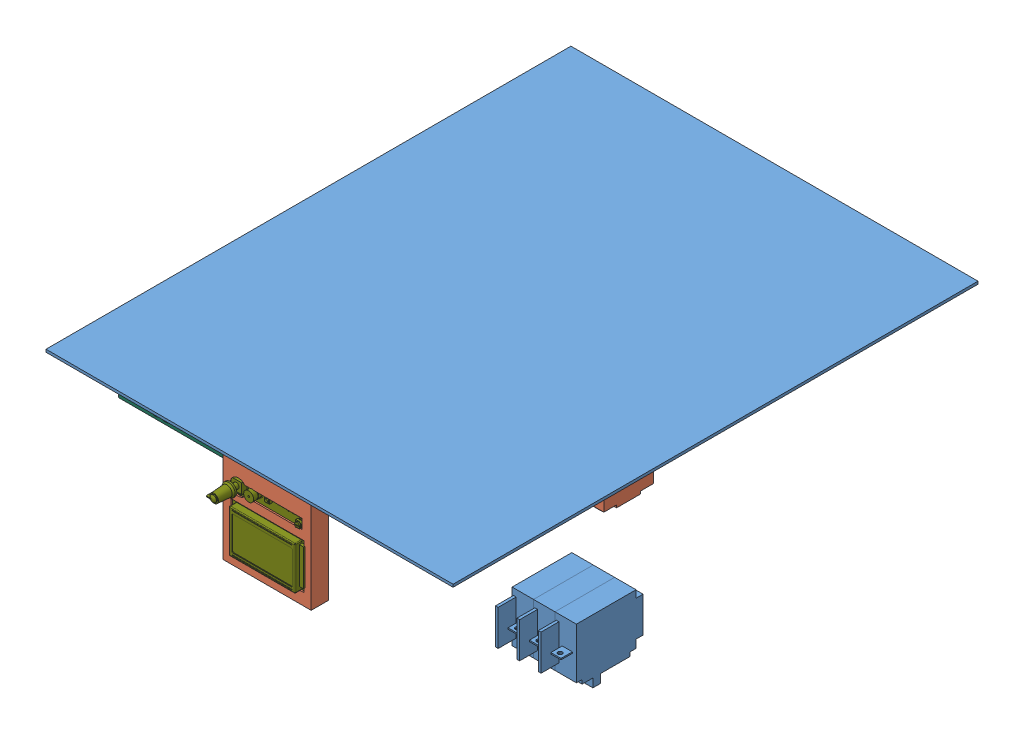
SolidWorks assembly CASE ASSEMBLY, configuration Default. Lengths in mm.
Overall size (670.4 210.09 685.13).
1343 component instances, 97 part files, 49 mates.
Components (placement in the parent):
- 24.5x24 sheet metal-1: 24.5x24 sheet metal [Default] at (-63.6847 2.1008 31.4018) size (482.6 3.17 622.3)
- SSR--H1.step-1: SSR--H1.step [Default] at (80.3153 -7.0742 117.6478) x (0 0 -1) z (-1 0 0) size (58.7 23.5 45.2)
- BIGTREETECH SKR 2-3D.step-2: BIGTREETECH SKR 2-3D.step [Default] at (122.8656 -8.0191 -250.7922) x (0 0 1) z (0 -1 0) size (112.33 85.75 22.11)
  - R51.step-1: R51.step [Default] at origin size (1.6 0.8 0.45)
    - R0603.step-1: R0603.step [Default] at (446.2816 199.1552 0) x (1 0 0) z (0 0 1) size (1.6 0.8 0.45)
  - D6.step-1: D6.step [Default] at origin size (1.25 2.02 1.1)
    - User_Library-led_0805.step-1: User_Library-led_0805.step [Default] at (466.0899 175.6538 0) x (0 1 0) z (0 0 1) size (2.02 1.25 1.1)
  - J26.step-1: J26.step [Default] at origin size (8 6 11)
    - User_Library-XH2_54_2PIN_RGB0.step-1: User_Library-XH2_54_2PIN_RGB0.step [Default] at (478.1261 231.8352 0) x (-1 0 0) z (0 1 0) size (8 11 6)
  - J25.step-1: J25.step [Default] at origin size (8 6 11)
    - User_Library-XH2_54_2PIN_RGB0.step-1: User_Library-XH2_54_2PIN_RGB0.step [Default] at (404.5931 231.8352 0) x (-1 0 0) z (0 1 0) size (8 11 6)
  - R91.step-1: R91.step [Default] at origin size (1.6 0.8 0.45)
    - R0603.step-1: R0603.step [Default] at (433.9497 171.3035 0) x (-1 0 0) z (0 0 1) size (1.6 0.8 0.45)
  - Q9.step-1: Q9.step [Default] at origin size (6.47 5 1.11)
    - lfpak.step-1: lfpak.step [Default] at (408.5301 152.605 0) x (0 1 0) z (1 0 0) size (5 1.11 6.47)
  - Q4.step-1: Q4.step [Default] at origin size (6.47 5 1.11)
    - lfpak.step-1: lfpak.step [Default] at (402.7151 191.195 0) x (0 1 0) z (1 0 0) size (5 1.11 6.47)
  - Q3.step-1: Q3.step [Default] at origin size (6.47 5 1.11)
    - lfpak.step-1: lfpak.step [Default] at (402.7961 199.786 0) x (0 1 0) z (1 0 0) size (5 1.11 6.47)
  - Q1.step-1: Q1.step [Default] at origin size (5 6.47 1.11)
    - lfpak.step-1: lfpak.step [Default] at (421.274 197.4849 0) x (1 0 0) z (0 -1 0) size (5 1.11 6.47)
  - J8.step-1: J8.step [Default] at origin size (10.18 5.84 7.5)
    - 810110576.step-1: 810110576.step [Default] at (471.763 164.5812 0) size (1.02 0.37 2.4)
      - Extruded.step-1: Extruded.step [Default] at origin size (1.02 0.37 2.4)
    - 810110712.step-1: 810110712.step [Default] at (474.8242 164.5862 0) size (5.11 0.36 6)
      - Extruded-0.step-1: Extruded-0.step [Default] at origin size (5.11 0.36 6)
    - 810110848.step-1: 810110848.step [Default] at (474.7241 161.8253 0) size (9.98 5.32 0.5)
      - Extruded-1.step-1: Extruded-1.step [Default] at origin size (9.98 5.32 0.5)
    - 810110984.step-1: 810110984.step [Default] at (474.8362 161.8472 0) size (10.16 5.84 6)
      - Extruded-2.step-1: Extruded-2.step [Default] at origin size (10.16 5.84 6)
    - 810111120.step-1: 810111120.step [Default] at (477.8853 164.5862 0) size (1.02 0.36 2.4)
      - Extruded-3.step-1: Extruded-3.step [Default] at origin size (1.02 0.36 2.4)
    - 860059712.step-1: 860059712.step [Default] at (477.384 162.2291 -1.5) x (0 1 0) z (0 0 1) size (1 1 6)
      - Cylinder.step-1: Cylinder.step [Default] at origin size (1 1 6)
    - 860059712.step-2: 860059712.step [Default] at (474.844 162.2291 -1.5) x (0 1 0) z (0 0 1) size (1 1 6)
      - Cylinder.step-1: Cylinder.step [Default] at origin size (1 1 6)
    - 860059712.step-3: 860059712.step [Default] at (472.304 162.2291 -1.5) x (0 1 0) z (0 0 1) size (1 1 6)
      - Cylinder.step-1: Cylinder.step [Default] at origin size (1 1 6)
  - J4.step-1: J4.step [Default] at origin size (5.84 10.18 7.5)
    - 810109760.step-1: 810109760.step [Default] at (474.5198 173.738 0) size (0.37 1.02 2.4)
      - Extruded-4.step-1: Extruded-4.step [Default] at origin size (0.37 1.02 2.4)
    - 810109896.step-1: 810109896.step [Default] at (474.5148 176.7991 0) size (0.36 5.11 6)
      - Extruded-5.step-1: Extruded-5.step [Default] at origin size (0.36 5.11 6)
    - 810110032.step-1: 810110032.step [Default] at (477.2757 176.6991 0) size (5.32 9.98 0.5)
      - Extruded-6.step-1: Extruded-6.step [Default] at origin size (5.32 9.98 0.5)
    - 810110168.step-1: 810110168.step [Default] at (477.2538 176.8112 0) size (5.84 10.16 6)
      - Extruded-7.step-1: Extruded-7.step [Default] at origin size (5.84 10.16 6)
    - 810110304.step-1: 810110304.step [Default] at (474.5148 179.8603 0) size (0.36 1.02 2.4)
      - Extruded-8.step-1: Extruded-8.step [Default] at origin size (0.36 1.02 2.4)
    - 860059456.step-1: 860059456.step [Default] at (476.8719 179.359 -1.5) x (-1 0 0) z (0 0 1) size (1 1 6)
      - Cylinder-9.step-1: Cylinder-9.step [Default] at origin size (1 1 6)
    - 860059456.step-2: 860059456.step [Default] at (476.8719 176.819 -1.5) x (-1 0 0) z (0 0 1) size (1 1 6)
      - Cylinder-9.step-1: Cylinder-9.step [Default] at origin size (1 1 6)
    - 860059456.step-3: 860059456.step [Default] at (476.8719 174.279 -1.5) x (-1 0 0) z (0 0 1) size (1 1 6)
      - Cylinder-9.step-1: Cylinder-9.step [Default] at origin size (1 1 6)
  - J3.step-1: J3.step [Default] at origin size (5.84 10.18 7.5)
    - 810109760.step-1: 810109760.step [Default] at (474.5198 184.288 0) size (0.37 1.02 2.4)
      - Extruded-4.step-1: Extruded-4.step [Default] at origin size (0.37 1.02 2.4)
    - 810109896.step-1: 810109896.step [Default] at (474.5148 187.3492 0) size (0.36 5.11 6)
      - Extruded-5.step-1: Extruded-5.step [Default] at origin size (0.36 5.11 6)
    - 810110032.step-1: 810110032.step [Default] at (477.2757 187.2491 0) size (5.32 9.98 0.5)
      - Extruded-6.step-1: Extruded-6.step [Default] at origin size (5.32 9.98 0.5)
    - 810110168.step-1: 810110168.step [Default] at (477.2538 187.3611 0) size (5.84 10.16 6)
      - Extruded-7.step-1: Extruded-7.step [Default] at origin size (5.84 10.16 6)
    - 810110304.step-1: 810110304.step [Default] at (474.5148 190.4103 0) size (0.36 1.02 2.4)
      - Extruded-8.step-1: Extruded-8.step [Default] at origin size (0.36 1.02 2.4)
    - 860059456.step-1: 860059456.step [Default] at (476.8719 189.909 -1.5) x (-1 0 0) z (0 0 1) size (1 1 6)
      - Cylinder-9.step-1: Cylinder-9.step [Default] at origin size (1 1 6)
    - 860059456.step-2: 860059456.step [Default] at (476.8719 187.369 -1.5) x (-1 0 0) z (0 0 1) size (1 1 6)
      - Cylinder-9.step-1: Cylinder-9.step [Default] at origin size (1 1 6)
    - 860059456.step-3: 860059456.step [Default] at (476.8719 184.829 -1.5) x (-1 0 0) z (0 0 1) size (1 1 6)
      - Cylinder-9.step-1: Cylinder-9.step [Default] at origin size (1 1 6)
  - J2.step-1: J2.step [Default] at origin size (5.84 10.18 7.5)
    - 810109760.step-1: 810109760.step [Default] at (474.5948 194.923 0) size (0.37 1.02 2.4)
      - Extruded-4.step-1: Extruded-4.step [Default] at origin size (0.37 1.02 2.4)
    - 810109896.step-1: 810109896.step [Default] at (474.5898 197.9841 0) size (0.36 5.11 6)
      - Extruded-5.step-1: Extruded-5.step [Default] at origin size (0.36 5.11 6)
    - 810110032.step-1: 810110032.step [Default] at (477.3507 197.884 0) size (5.32 9.98 0.5)
      - Extruded-6.step-1: Extruded-6.step [Default] at origin size (5.32 9.98 0.5)
    - 810110168.step-1: 810110168.step [Default] at (477.3288 197.9962 0) size (5.84 10.16 6)
      - Extruded-7.step-1: Extruded-7.step [Default] at origin size (5.84 10.16 6)
    - 810110304.step-1: 810110304.step [Default] at (474.5898 201.0453 0) size (0.36 1.02 2.4)
      - Extruded-8.step-1: Extruded-8.step [Default] at origin size (0.36 1.02 2.4)
    - 860059456.step-1: 860059456.step [Default] at (476.9469 200.544 -1.5) x (-1 0 0) z (0 0 1) size (1 1 6)
      - Cylinder-9.step-1: Cylinder-9.step [Default] at origin size (1 1 6)
    - 860059456.step-2: 860059456.step [Default] at (476.9469 198.004 -1.5) x (-1 0 0) z (0 0 1) size (1 1 6)
      - Cylinder-9.step-1: Cylinder-9.step [Default] at origin size (1 1 6)
    - 860059456.step-3: 860059456.step [Default] at (476.9469 195.464 -1.5) x (-1 0 0) z (0 0 1) size (1 1 6)
      - Cylinder-9.step-1: Cylinder-9.step [Default] at origin size (1 1 6)
  - C11.step-1: C11.step [Default] at origin size (0.8 1.6 0.8)
    - 810109080.step-1: 810109080.step [Default] at (447.0486 175.6409 0) size (0.8 0.23 0.8)
      - Extruded-10.step-1: Extruded-10.step [Default] at origin size (0.8 0.23 0.8)
    - 810109080.step-2: 810109080.step [Default] at (447.0486 177.0109 0) size (0.8 0.23 0.8)
      - Extruded-10.step-1: Extruded-10.step [Default] at origin size (0.8 0.23 0.8)
    - 810109216.step-1: 810109216.step [Default] at (447.0487 176.3259 0) size (0.8 1.14 0.8)
      - Extruded-11.step-1: Extruded-11.step [Default] at origin size (0.8 1.14 0.8)
  - R2.step-1: R2.step [Default] at origin size (1.6 0.8 0.45)
    - R0603.step-1: R0603.step [Default] at (470.8993 199.0332 0) x (1 0 0) z (0 0 1) size (1.6 0.8 0.45)
  - R1.step-1: R1.step [Default] at origin size (1.6 0.8 0.45)
    - R0603.step-1: R0603.step [Default] at (470.8993 197.5092 0) x (1 0 0) z (0 0 1) size (1.6 0.8 0.45)
  - R9.step-1: R9.step [Default] at origin size (1.6 0.8 0.45)
    - R0603.step-1: R0603.step [Default] at (470.8993 194.4612 0) x (1 0 0) z (0 0 1) size (1.6 0.8 0.45)
  - R8.step-1: R8.step [Default] at origin size (1.6 0.8 0.45)
    - R0603.step-1: R0603.step [Default] at (470.8993 195.9852 0) x (1 0 0) z (0 0 1) size (1.6 0.8 0.45)
  - R15.step-1: R15.step [Default] at origin size (1.6 0.8 0.45)
    - R0603.step-1: R0603.step [Default] at (439.148 184.8042 0) x (1 0 0) z (0 0 1) size (1.6 0.8 0.45)
  - R20.step-1: R20.step [Default] at origin size (1.6 0.8 0.45)
    - R0603.step-1: R0603.step [Default] at (470.9086 173.1202 0) x (1 0 0) z (0 0 1) size (1.6 0.8 0.45)
  - Z-CLS.step-1: Z-CLS.step [Default] at origin size (15.24 2.54 11.54)
    - 1001-6.step-1: 1001-6.step [Default] at (452.256 205.359 0) x (-1 0 0) z (0 0 1) size (15.24 2.54 11.54)
  - Y-CLS.step-1: Y-CLS.step [Default] at origin size (15.24 2.54 11.54)
    - 1001-6.step-1: 1001-6.step [Default] at (436.127 205.359 0) x (-1 0 0) z (0 0 1) size (15.24 2.54 11.54)
  - X-CLS.step-1: X-CLS.step [Default] at origin size (15.24 2.54 11.54)
    - 1001-6.step-1: 1001-6.step [Default] at (419.998 205.359 0) x (-1 0 0) z (0 0 1) size (15.24 2.54 11.54)
  - E1-CLS.step-1: E1-CLS.step [Default] at origin size (15.24 2.54 11.54)
    - 1001-6.step-1: 1001-6.step [Default] at (484.641 205.359 0) x (-1 0 0) z (0 0 1) size (15.24 2.54 11.54)
  - E0-CLS.step-1: E0-CLS.step [Default] at origin size (15.24 2.54 11.54)
    - 1001-6.step-1: 1001-6.step [Default] at (468.512 205.359 0) x (-1 0 0) z (0 0 1) size (15.24 2.54 11.54)
  - ZSPI1.step-1: ZSPI1.step [Default] at origin size (5.08 10.16 11.54)
    - 1001-4.step-1: 1001-4.step [Default] at (450.14 220.535 0) x (0 -1 0) z (0 0 1) size (10.16 2.54 11.54)
    - 1001-4.step-2: 1001-4.step [Default] at (447.6 220.536 0) x (0 -1 0) z (0 0 1) size (10.16 2.54 11.54)
  - ZMS1.step-1: ZMS1.step [Default] at origin size (2.54 10.16 11.54)
    - 1001-4.step-1: 1001-4.step [Default] at (452.675 212.915 0) x (0 1 0) z (0 0 1) size (10.16 2.54 11.54)
  - ZMB.step-1: ZMB.step [Default] at origin size (12.7 5.85 7.5)
    - 810111256.step-1: 810111256.step [Default] at (450.5983 228.8308 0) size (12.7 5.84 6)
      - Extruded-12.step-1: Extruded-12.step [Default] at origin size (12.7 5.84 6)
    - 810110576.step-1: 810110576.step [Default] at (446.2907 231.5753 0) size (1.02 0.37 2.4)
      - Extruded.step-1: Extruded.step [Default] at origin size (1.02 0.37 2.4)
    - 810111120.step-1: 810111120.step [Default] at (454.9267 231.5803 0) size (1.02 0.36 2.4)
      - Extruded-3.step-1: Extruded-3.step [Default] at origin size (1.02 0.36 2.4)
    - 810111392.step-1: 810111392.step [Default] at (450.5706 231.5803 0) size (7.62 0.36 6)
      - Extruded-13.step-1: Extruded-13.step [Default] at origin size (7.62 0.36 6)
    - 810111528.step-1: 810111528.step [Default] at (450.6341 228.8089 0) size (12.22 5.32 0.5)
      - Extruded-14.step-1: Extruded-14.step [Default] at origin size (12.22 5.32 0.5)
    - 860059712.step-1: 860059712.step [Default] at (446.795 229.2127 -1.5) x (0 1 0) z (0 0 1) size (1 1 6)
      - Cylinder.step-1: Cylinder.step [Default] at origin size (1 1 6)
    - 860059712.step-2: 860059712.step [Default] at (449.335 229.2127 -1.5) x (0 1 0) z (0 0 1) size (1 1 6)
      - Cylinder.step-1: Cylinder.step [Default] at origin size (1 1 6)
    - 860059712.step-3: 860059712.step [Default] at (451.875 229.2127 -1.5) x (0 1 0) z (0 0 1) size (1 1 6)
      - Cylinder.step-1: Cylinder.step [Default] at origin size (1 1 6)
    - 860059712.step-4: 860059712.step [Default] at (454.415 229.2127 -1.5) x (0 1 0) z (0 0 1) size (1 1 6)
      - Cylinder.step-1: Cylinder.step [Default] at origin size (1 1 6)
  - ZMA.step-1: ZMA.step [Default] at origin size (12.7 5.85 7.5)
    - 810111256.step-1: 810111256.step [Default] at (437.3903 228.8308 0) size (12.7 5.84 6)
      - Extruded-12.step-1: Extruded-12.step [Default] at origin size (12.7 5.84 6)
    - 810110576.step-1: 810110576.step [Default] at (433.0827 231.5753 0) size (1.02 0.37 2.4)
      - Extruded.step-1: Extruded.step [Default] at origin size (1.02 0.37 2.4)
    - 810111120.step-1: 810111120.step [Default] at (441.7187 231.5803 0) size (1.02 0.36 2.4)
      - Extruded-3.step-1: Extruded-3.step [Default] at origin size (1.02 0.36 2.4)
    - 810111392.step-1: 810111392.step [Default] at (437.3626 231.5803 0) size (7.62 0.36 6)
      - Extruded-13.step-1: Extruded-13.step [Default] at origin size (7.62 0.36 6)
    - 810111528.step-1: 810111528.step [Default] at (437.4261 228.8089 0) size (12.22 5.32 0.5)
      - Extruded-14.step-1: Extruded-14.step [Default] at origin size (12.22 5.32 0.5)
    - 860059712.step-1: 860059712.step [Default] at (433.587 229.2127 -1.5) x (0 1 0) z (0 0 1) size (1 1 6)
      - Cylinder.step-1: Cylinder.step [Default] at origin size (1 1 6)
    - 860059712.step-2: 860059712.step [Default] at (436.127 229.2127 -1.5) x (0 1 0) z (0 0 1) size (1 1 6)
      - Cylinder.step-1: Cylinder.step [Default] at origin size (1 1 6)
    - 860059712.step-3: 860059712.step [Default] at (438.667 229.2127 -1.5) x (0 1 0) z (0 0 1) size (1 1 6)
      - Cylinder.step-1: Cylinder.step [Default] at origin size (1 1 6)
    - 860059712.step-4: 860059712.step [Default] at (441.207 229.2127 -1.5) x (0 1 0) z (0 0 1) size (1 1 6)
      - Cylinder.step-1: Cylinder.step [Default] at origin size (1 1 6)
  - ZDR1.step-1: ZDR1.step [Default] at origin size (20.32 15.24 8.51)
    - 810111664.step-1: 810111664.step [Default] at (443.9793 210.3755 0) size (20.32 2.54 8.5)
      - Extruded-15.step-1: Extruded-15.step [Default] at origin size (20.32 2.54 8.5)
    - 810109352.step-1: 810109352.step [Default] at (452.8693 210.3755 8.5) size (1.6 1.6 0.01)
      - Extruded-16.step-1: Extruded-16.step [Default] at origin size (1.6 1.6 0.01)
    - 810109352.step-2: 810109352.step [Default] at (450.3293 210.3755 8.5) size (1.6 1.6 0.01)
      - Extruded-16.step-1: Extruded-16.step [Default] at origin size (1.6 1.6 0.01)
    - 810109352.step-3: 810109352.step [Default] at (447.7893 210.3755 8.5) size (1.6 1.6 0.01)
      - Extruded-16.step-1: Extruded-16.step [Default] at origin size (1.6 1.6 0.01)
    - 810109352.step-4: 810109352.step [Default] at (445.2493 210.3755 8.5) size (1.6 1.6 0.01)
      - Extruded-16.step-1: Extruded-16.step [Default] at origin size (1.6 1.6 0.01)
    - 810109352.step-5: 810109352.step [Default] at (442.7093 210.3755 8.5) size (1.6 1.6 0.01)
      - Extruded-16.step-1: Extruded-16.step [Default] at origin size (1.6 1.6 0.01)
    - 810109352.step-6: 810109352.step [Default] at (440.1693 210.3755 8.5) size (1.6 1.6 0.01)
      - Extruded-16.step-1: Extruded-16.step [Default] at origin size (1.6 1.6 0.01)
    - 810109352.step-7: 810109352.step [Default] at (437.6293 210.3755 8.5) size (1.6 1.6 0.01)
      - Extruded-16.step-1: Extruded-16.step [Default] at origin size (1.6 1.6 0.01)
    - 810109352.step-8: 810109352.step [Default] at (435.0893 210.3755 8.5) size (1.6 1.6 0.01)
      - Extruded-16.step-1: Extruded-16.step [Default] at origin size (1.6 1.6 0.01)
    - 810111800.step-1: 810111800.step [Default] at (443.9793 223.0755 0) size (20.32 2.54 8.5)
      - Extruded-17.step-1: Extruded-17.step [Default] at origin size (20.32 2.54 8.5)
    - 810109352.step-9: 810109352.step [Default] at (435.0893 223.0755 8.5) size (1.6 1.6 0.01)
      - Extruded-16.step-1: Extruded-16.step [Default] at origin size (1.6 1.6 0.01)
    - 810109352.step-10: 810109352.step [Default] at (437.6293 223.0755 8.5) size (1.6 1.6 0.01)
      - Extruded-16.step-1: Extruded-16.step [Default] at origin size (1.6 1.6 0.01)
    - 810109352.step-11: 810109352.step [Default] at (440.1693 223.0755 8.5) size (1.6 1.6 0.01)
      - Extruded-16.step-1: Extruded-16.step [Default] at origin size (1.6 1.6 0.01)
    - 810109352.step-12: 810109352.step [Default] at (442.7093 223.0755 8.5) size (1.6 1.6 0.01)
      - Extruded-16.step-1: Extruded-16.step [Default] at origin size (1.6 1.6 0.01)
    - 810109352.step-13: 810109352.step [Default] at (445.2493 223.0755 8.5) size (1.6 1.6 0.01)
      - Extruded-16.step-1: Extruded-16.step [Default] at origin size (1.6 1.6 0.01)
    - 810109352.step-14: 810109352.step [Default] at (447.7893 223.0755 8.5) size (1.6 1.6 0.01)
      - Extruded-16.step-1: Extruded-16.step [Default] at origin size (1.6 1.6 0.01)
    - 810109352.step-15: 810109352.step [Default] at (450.3293 223.0755 8.5) size (1.6 1.6 0.01)
      - Extruded-16.step-1: Extruded-16.step [Default] at origin size (1.6 1.6 0.01)
    - 810109352.step-16: 810109352.step [Default] at (452.8693 223.0755 8.5) size (1.6 1.6 0.01)
      - Extruded-16.step-1: Extruded-16.step [Default] at origin size (1.6 1.6 0.01)
    - 810111936.step-1: 810111936.step [Default] at (435.0893 214.2617 0) size (2.54 4.93 8.5)
      - Extruded-18.step-1: Extruded-18.step [Default] at origin size (2.54 4.93 8.5)
    - 810109352.step-17: 810109352.step [Default] at (435.0893 212.9155 8.5) size (1.6 1.6 0.01)
      - Extruded-16.step-1: Extruded-16.step [Default] at origin size (1.6 1.6 0.01)
    - 810109352.step-18: 810109352.step [Default] at (435.0893 215.4555 8.5) size (1.6 1.6 0.01)
      - Extruded-16.step-1: Extruded-16.step [Default] at origin size (1.6 1.6 0.01)
  - YSPI1.step-1: YSPI1.step [Default] at origin size (5.08 10.16 11.54)
    - 1001-4.step-1: 1001-4.step [Default] at (428.5 220.535 0) x (0 -1 0) z (0 0 1) size (10.16 2.54 11.54)
    - 1001-4.step-2: 1001-4.step [Default] at (425.96 220.536 0) x (0 -1 0) z (0 0 1) size (10.16 2.54 11.54)
  - YM.step-1: YM.step [Default] at origin size (12.7 5.85 7.5)
    - 810111256.step-1: 810111256.step [Default] at (424.1823 228.8308 0) size (12.7 5.84 6)
      - Extruded-12.step-1: Extruded-12.step [Default] at origin size (12.7 5.84 6)
    - 810110576.step-1: 810110576.step [Default] at (419.8747 231.5753 0) size (1.02 0.37 2.4)
      - Extruded.step-1: Extruded.step [Default] at origin size (1.02 0.37 2.4)
    - 810111120.step-1: 810111120.step [Default] at (428.5107 231.5803 0) size (1.02 0.36 2.4)
      - Extruded-3.step-1: Extruded-3.step [Default] at origin size (1.02 0.36 2.4)
    - 810111392.step-1: 810111392.step [Default] at (424.1546 231.5803 0) size (7.62 0.36 6)
      - Extruded-13.step-1: Extruded-13.step [Default] at origin size (7.62 0.36 6)
    - 810111528.step-1: 810111528.step [Default] at (424.2181 228.8089 0) size (12.22 5.32 0.5)
      - Extruded-14.step-1: Extruded-14.step [Default] at origin size (12.22 5.32 0.5)
    - 860059712.step-1: 860059712.step [Default] at (420.379 229.2127 -1.5) x (0 1 0) z (0 0 1) size (1 1 6)
      - Cylinder.step-1: Cylinder.step [Default] at origin size (1 1 6)
    - 860059712.step-2: 860059712.step [Default] at (422.919 229.2127 -1.5) x (0 1 0) z (0 0 1) size (1 1 6)
      - Cylinder.step-1: Cylinder.step [Default] at origin size (1 1 6)
    - 860059712.step-3: 860059712.step [Default] at (425.459 229.2127 -1.5) x (0 1 0) z (0 0 1) size (1 1 6)
      - Cylinder.step-1: Cylinder.step [Default] at origin size (1 1 6)
    - 860059712.step-4: 860059712.step [Default] at (427.999 229.2127 -1.5) x (0 1 0) z (0 0 1) size (1 1 6)
      - Cylinder.step-1: Cylinder.step [Default] at origin size (1 1 6)
  - YMS1.step-1: YMS1.step [Default] at origin size (2.54 10.16 11.54)
    - 1001-4.step-1: 1001-4.step [Default] at (431.05 212.915 0) x (0 1 0) z (0 0 1) size (10.16 2.54 11.54)
  - YDR1.step-1: YDR1.step [Default] at origin size (20.32 15.24 8.51)
    - 810111664.step-1: 810111664.step [Default] at (422.3512 210.3755 0) size (20.32 2.54 8.5)
      - Extruded-15.step-1: Extruded-15.step [Default] at origin size (20.32 2.54 8.5)
    - 810109352.step-1: 810109352.step [Default] at (431.2412 210.3755 8.5) size (1.6 1.6 0.01)
      - Extruded-16.step-1: Extruded-16.step [Default] at origin size (1.6 1.6 0.01)
    - 810109352.step-2: 810109352.step [Default] at (428.7012 210.3755 8.5) size (1.6 1.6 0.01)
      - Extruded-16.step-1: Extruded-16.step [Default] at origin size (1.6 1.6 0.01)
    - 810109352.step-3: 810109352.step [Default] at (426.1612 210.3755 8.5) size (1.6 1.6 0.01)
      - Extruded-16.step-1: Extruded-16.step [Default] at origin size (1.6 1.6 0.01)
    - 810109352.step-4: 810109352.step [Default] at (423.6212 210.3755 8.5) size (1.6 1.6 0.01)
      - Extruded-16.step-1: Extruded-16.step [Default] at origin size (1.6 1.6 0.01)
    - 810109352.step-5: 810109352.step [Default] at (421.0812 210.3755 8.5) size (1.6 1.6 0.01)
      - Extruded-16.step-1: Extruded-16.step [Default] at origin size (1.6 1.6 0.01)
    - 810109352.step-6: 810109352.step [Default] at (418.5412 210.3755 8.5) size (1.6 1.6 0.01)
      - Extruded-16.step-1: Extruded-16.step [Default] at origin size (1.6 1.6 0.01)
    - 810109352.step-7: 810109352.step [Default] at (416.0012 210.3755 8.5) size (1.6 1.6 0.01)
      - Extruded-16.step-1: Extruded-16.step [Default] at origin size (1.6 1.6 0.01)
    - 810109352.step-8: 810109352.step [Default] at (413.4612 210.3755 8.5) size (1.6 1.6 0.01)
      - Extruded-16.step-1: Extruded-16.step [Default] at origin size (1.6 1.6 0.01)
    - 810111800.step-1: 810111800.step [Default] at (422.3512 223.0755 0) size (20.32 2.54 8.5)
      - Extruded-17.step-1: Extruded-17.step [Default] at origin size (20.32 2.54 8.5)
    - 810109352.step-9: 810109352.step [Default] at (413.4612 223.0755 8.5) size (1.6 1.6 0.01)
      - Extruded-16.step-1: Extruded-16.step [Default] at origin size (1.6 1.6 0.01)
    - 810109352.step-10: 810109352.step [Default] at (416.0012 223.0755 8.5) size (1.6 1.6 0.01)
      - Extruded-16.step-1: Extruded-16.step [Default] at origin size (1.6 1.6 0.01)
    - 810109352.step-11: 810109352.step [Default] at (418.5412 223.0755 8.5) size (1.6 1.6 0.01)
      - Extruded-16.step-1: Extruded-16.step [Default] at origin size (1.6 1.6 0.01)
    - 810109352.step-12: 810109352.step [Default] at (421.0812 223.0755 8.5) size (1.6 1.6 0.01)
      - Extruded-16.step-1: Extruded-16.step [Default] at origin size (1.6 1.6 0.01)
    - 810109352.step-13: 810109352.step [Default] at (423.6212 223.0755 8.5) size (1.6 1.6 0.01)
      - Extruded-16.step-1: Extruded-16.step [Default] at origin size (1.6 1.6 0.01)
    - 810109352.step-14: 810109352.step [Default] at (426.1612 223.0755 8.5) size (1.6 1.6 0.01)
      - Extruded-16.step-1: Extruded-16.step [Default] at origin size (1.6 1.6 0.01)
    - 810109352.step-15: 810109352.step [Default] at (428.7012 223.0755 8.5) size (1.6 1.6 0.01)
      - Extruded-16.step-1: Extruded-16.step [Default] at origin size (1.6 1.6 0.01)
    - 810109352.step-16: 810109352.step [Default] at (431.2412 223.0755 8.5) size (1.6 1.6 0.01)
      - Extruded-16.step-1: Extruded-16.step [Default] at origin size (1.6 1.6 0.01)
    - 810111936.step-1: 810111936.step [Default] at (413.4612 214.2617 0) size (2.54 4.93 8.5)
      - Extruded-18.step-1: Extruded-18.step [Default] at origin size (2.54 4.93 8.5)
    - 810109352.step-17: 810109352.step [Default] at (413.4612 212.9155 8.5) size (1.6 1.6 0.01)
      - Extruded-16.step-1: Extruded-16.step [Default] at origin size (1.6 1.6 0.01)
    - 810109352.step-18: 810109352.step [Default] at (413.4612 215.4555 8.5) size (1.6 1.6 0.01)
      - Extruded-16.step-1: Extruded-16.step [Default] at origin size (1.6 1.6 0.01)
  - XSPI1.step-1: XSPI1.step [Default] at origin size (5.08 10.16 11.54)
    - 1001-4.step-1: 1001-4.step [Default] at (406.85 220.535 0) x (0 -1 0) z (0 0 1) size (10.16 2.54 11.54)
    - 1001-4.step-2: 1001-4.step [Default] at (404.31 220.536 0) x (0 -1 0) z (0 0 1) size (10.16 2.54 11.54)
  - XM.step-1: XM.step [Default] at origin size (12.7 5.85 7.5)
    - 810111256.step-1: 810111256.step [Default] at (410.9743 228.8308 0) size (12.7 5.84 6)
      - Extruded-12.step-1: Extruded-12.step [Default] at origin size (12.7 5.84 6)
    - 810110576.step-1: 810110576.step [Default] at (406.6667 231.5753 0) size (1.02 0.37 2.4)
      - Extruded.step-1: Extruded.step [Default] at origin size (1.02 0.37 2.4)
    - 810111120.step-1: 810111120.step [Default] at (415.3027 231.5803 0) size (1.02 0.36 2.4)
      - Extruded-3.step-1: Extruded-3.step [Default] at origin size (1.02 0.36 2.4)
    - 810111392.step-1: 810111392.step [Default] at (410.9466 231.5803 0) size (7.62 0.36 6)
      - Extruded-13.step-1: Extruded-13.step [Default] at origin size (7.62 0.36 6)
    - 810111528.step-1: 810111528.step [Default] at (411.0101 228.8089 0) size (12.22 5.32 0.5)
      - Extruded-14.step-1: Extruded-14.step [Default] at origin size (12.22 5.32 0.5)
    - 860059712.step-1: 860059712.step [Default] at (407.171 229.2127 -1.5) x (0 1 0) z (0 0 1) size (1 1 6)
      - Cylinder.step-1: Cylinder.step [Default] at origin size (1 1 6)
    - 860059712.step-2: 860059712.step [Default] at (409.711 229.2127 -1.5) x (0 1 0) z (0 0 1) size (1 1 6)
      - Cylinder.step-1: Cylinder.step [Default] at origin size (1 1 6)
    - 860059712.step-3: 860059712.step [Default] at (412.251 229.2127 -1.5) x (0 1 0) z (0 0 1) size (1 1 6)
      - Cylinder.step-1: Cylinder.step [Default] at origin size (1 1 6)
    - 860059712.step-4: 860059712.step [Default] at (414.791 229.2127 -1.5) x (0 1 0) z (0 0 1) size (1 1 6)
      - Cylinder.step-1: Cylinder.step [Default] at origin size (1 1 6)
  - XMS1.step-1: XMS1.step [Default] at origin size (2.54 10.16 11.54)
    - 1001-4.step-1: 1001-4.step [Default] at (409.4 212.915 0) x (0 1 0) z (0 0 1) size (10.16 2.54 11.54)
  - XDR1.step-1: XDR1.step [Default] at origin size (20.32 15.24 8.51)
    - 810111664.step-1: 810111664.step [Default] at (400.7104 210.3755 0) size (20.32 2.54 8.5)
      - Extruded-15.step-1: Extruded-15.step [Default] at origin size (20.32 2.54 8.5)
    - 810109352.step-1: 810109352.step [Default] at (409.6004 210.3755 8.5) size (1.6 1.6 0.01)
      - Extruded-16.step-1: Extruded-16.step [Default] at origin size (1.6 1.6 0.01)
    - 810109352.step-2: 810109352.step [Default] at (407.0604 210.3755 8.5) size (1.6 1.6 0.01)
      - Extruded-16.step-1: Extruded-16.step [Default] at origin size (1.6 1.6 0.01)
    - 810109352.step-3: 810109352.step [Default] at (404.5204 210.3755 8.5) size (1.6 1.6 0.01)
      - Extruded-16.step-1: Extruded-16.step [Default] at origin size (1.6 1.6 0.01)
    - 810109352.step-4: 810109352.step [Default] at (401.9804 210.3755 8.5) size (1.6 1.6 0.01)
      - Extruded-16.step-1: Extruded-16.step [Default] at origin size (1.6 1.6 0.01)
    - 810109352.step-5: 810109352.step [Default] at (399.4404 210.3755 8.5) size (1.6 1.6 0.01)
      - Extruded-16.step-1: Extruded-16.step [Default] at origin size (1.6 1.6 0.01)
    - 810109352.step-6: 810109352.step [Default] at (396.9004 210.3755 8.5) size (1.6 1.6 0.01)
      - Extruded-16.step-1: Extruded-16.step [Default] at origin size (1.6 1.6 0.01)
    - 810109352.step-7: 810109352.step [Default] at (394.3604 210.3755 8.5) size (1.6 1.6 0.01)
      - Extruded-16.step-1: Extruded-16.step [Default] at origin size (1.6 1.6 0.01)
    - 810109352.step-8: 810109352.step [Default] at (391.8204 210.3755 8.5) size (1.6 1.6 0.01)
      - Extruded-16.step-1: Extruded-16.step [Default] at origin size (1.6 1.6 0.01)
    - 810111800.step-1: 810111800.step [Default] at (400.7104 223.0755 0) size (20.32 2.54 8.5)
      - Extruded-17.step-1: Extruded-17.step [Default] at origin size (20.32 2.54 8.5)
    - 810109352.step-9: 810109352.step [Default] at (391.8204 223.0755 8.5) size (1.6 1.6 0.01)
      - Extruded-16.step-1: Extruded-16.step [Default] at origin size (1.6 1.6 0.01)
    - 810109352.step-10: 810109352.step [Default] at (394.3604 223.0755 8.5) size (1.6 1.6 0.01)
      - Extruded-16.step-1: Extruded-16.step [Default] at origin size (1.6 1.6 0.01)
    - 810109352.step-11: 810109352.step [Default] at (396.9004 223.0755 8.5) size (1.6 1.6 0.01)
      - Extruded-16.step-1: Extruded-16.step [Default] at origin size (1.6 1.6 0.01)
    - 810109352.step-12: 810109352.step [Default] at (399.4404 223.0755 8.5) size (1.6 1.6 0.01)
      - Extruded-16.step-1: Extruded-16.step [Default] at origin size (1.6 1.6 0.01)
    - 810109352.step-13: 810109352.step [Default] at (401.9804 223.0755 8.5) size (1.6 1.6 0.01)
      - Extruded-16.step-1: Extruded-16.step [Default] at origin size (1.6 1.6 0.01)
    - 810109352.step-14: 810109352.step [Default] at (404.5204 223.0755 8.5) size (1.6 1.6 0.01)
      - Extruded-16.step-1: Extruded-16.step [Default] at origin size (1.6 1.6 0.01)
    - 810109352.step-15: 810109352.step [Default] at (407.0604 223.0755 8.5) size (1.6 1.6 0.01)
      - Extruded-16.step-1: Extruded-16.step [Default] at origin size (1.6 1.6 0.01)
    - 810109352.step-16: 810109352.step [Default] at (409.6004 223.0755 8.5) size (1.6 1.6 0.01)
      - Extruded-16.step-1: Extruded-16.step [Default] at origin size (1.6 1.6 0.01)
    - 810111936.step-1: 810111936.step [Default] at (391.8204 214.2617 0) size (2.54 4.93 8.5)
      - Extruded-18.step-1: Extruded-18.step [Default] at origin size (2.54 4.93 8.5)
    - 810109352.step-17: 810109352.step [Default] at (391.8204 212.9155 8.5) size (1.6 1.6 0.01)
      - Extruded-16.step-1: Extruded-16.step [Default] at origin size (1.6 1.6 0.01)
    - 810109352.step-18: 810109352.step [Default] at (391.8204 215.4555 8.5) size (1.6 1.6 0.01)
      - Extruded-16.step-1: Extruded-16.step [Default] at origin size (1.6 1.6 0.01)
  - U3.step-1: U3.step [Default] at origin size (6.5 6.96 1.7)
    - SOT-223_MP04A.step-1: SOT-223_MP04A.step [Default] at (443.155 169.8244 0) x (-1 0 0) z (0 0 1) size (6.5 6.96 1.7)
  - U2.step-1: U2.step [Default] at origin size (2.8 2.9 1.2)
    - SOT-23-5.step-1: SOT-23-5.step [Default] at (461.1879 167.132 0) x (0 -1 0) z (0 0 1) size (2.9 2.8 1.2)
  - R77.step-1: R77.step [Default] at origin size (0.8 1.6 0.45)
    - R0603.step-1: R0603.step [Default] at (439.8138 162.8147 0) x (0 -1 0) z (0 0 1) size (1.6 0.8 0.45)
  - R74.step-1: R74.step [Default] at origin size (0.8 1.6 0.45)
    - R0603.step-1: R0603.step [Default] at (438.3026 162.8147 0) x (0 -1 0) z (0 0 1) size (1.6 0.8 0.45)
  - R72.step-1: R72.step [Default] at origin size (0.8 1.6 0.45)
    - R0603.step-1: R0603.step [Default] at (441.3506 162.8147 0) x (0 -1 0) z (0 0 1) size (1.6 0.8 0.45)
  - R69.step-1: R69.step [Default] at origin size (0.8 1.6 0.45)
    - R0603.step-1: R0603.step [Default] at (433.7306 162.8147 0) x (0 -1 0) z (0 0 1) size (1.6 0.8 0.45)
  - R66.step-1: R66.step [Default] at origin size (1.6 0.8 0.45)
    - R0603.step-1: R0603.step [Default] at (439.6873 212.6942 0) x (1 0 0) z (0 0 1) size (1.6 0.8 0.45)
  - R68.step-1: R68.step [Default] at origin size (1.6 0.8 0.45)
    - R0603.step-1: R0603.step [Default] at (490.0923 162.1918 0) x (1 0 0) z (0 0 1) size (1.6 0.8 0.45)
  - R67.step-1: R67.step [Default] at origin size (1.6 0.8 0.45)
    - R0603.step-1: R0603.step [Default] at (490.0923 160.6678 0) x (1 0 0) z (0 0 1) size (1.6 0.8 0.45)
  - R65.step-1: R65.step [Default] at origin size (1.6 0.8 0.45)
    - R0603.step-1: R0603.step [Default] at (443.6117 163.5632 0) x (-1 0 0) z (0 0 1) size (1.6 0.8 0.45)
  - R33.step-1: R33.step [Default] at origin size (0.8 1.6 0.45)
    - R0603.step-1: R0603.step [Default] at (464.5404 175.6724 0) x (0 1 0) z (0 0 1) size (1.6 0.8 0.45)
  - R43.step-1: R43.step [Default] at origin size (1.6 0.8 0.45)
    - R0603.step-1: R0603.step [Default] at (418.0123 212.6942 0) x (1 0 0) z (0 0 1) size (1.6 0.8 0.45)
  - R28.step-1: R28.step [Default] at origin size (1.6 0.8 0.45)
    - R0603.step-1: R0603.step [Default] at (396.3873 212.6942 0) x (1 0 0) z (0 0 1) size (1.6 0.8 0.45)
  - R25.step-1: R25.step [Default] at origin size (1.6 0.8 0.45)
    - R0603.step-1: R0603.step [Default] at (490.0177 159.1055 0) x (-1 0 0) z (0 0 1) size (1.6 0.8 0.45)
  - R17.step-1: R17.step [Default] at origin size (1.6 0.8 0.45)
    - R0603.step-1: R0603.step [Default] at (461.3623 212.6942 0) x (1 0 0) z (0 0 1) size (1.6 0.8 0.45)
  - R14.step-1: R14.step [Default] at origin size (0.8 1.6 0.45)
    - R0603.step-1: R0603.step [Default] at (458.0515 167.1643 0) x (0 1 0) z (0 0 1) size (1.6 0.8 0.45)
  - R11.step-1: R11.step [Default] at origin size (1.6 0.8 0.45)
    - R0603.step-1: R0603.step [Default] at (470.8993 185.2882 0) x (1 0 0) z (0 0 1) size (1.6 0.8 0.45)
  - R10.step-1: R10.step [Default] at origin size (1.6 0.8 0.45)
    - R0603.step-1: R0603.step [Default] at (470.8993 186.8122 0) x (1 0 0) z (0 0 1) size (1.6 0.8 0.45)
  - R7.step-1: R7.step [Default] at origin size (1.6 0.8 0.45)
    - R0603.step-1: R0603.step [Default] at (470.8993 179.2652 0) x (1 0 0) z (0 0 1) size (1.6 0.8 0.45)
  - R6.step-1: R6.step [Default] at origin size (1.6 0.8 0.45)
    - R0603.step-1: R0603.step [Default] at (470.8993 177.7475 0) x (1 0 0) z (0 0 1) size (1.6 0.8 0.45)
  - R5.step-1: R5.step [Default] at origin size (1.6 0.8 0.45)
    - R0603.step-1: R0603.step [Default] at (470.8993 189.8622 0) x (1 0 0) z (0 0 1) size (1.6 0.8 0.45)
  - R4.step-1: R4.step [Default] at origin size (1.6 0.8 0.45)
    - R0603.step-1: R0603.step [Default] at (470.8993 188.3445 0) x (1 0 0) z (0 0 1) size (1.6 0.8 0.45)
  - R3.step-1: R3.step [Default] at origin size (1.6 0.8 0.45)
    - R0603.step-1: R0603.step [Default] at (482.9873 212.6942 0) x (1 0 0) z (0 0 1) size (1.6 0.8 0.45)
  - J18.step-1: J18.step [Default] at origin size (15.12 16.3 14.22)
    - USB-B-S-F-B-TH.step-1: USB-B-S-F-B-TH.step [Default] at (419.3379 154.6083 5.3) x (1 0 0) z (0 -1 0) size (15.12 14.22 16.3)
  - J16.step-1: J16.step [Default] at origin size (10.3 10.6 17.95)
    - KF128.step-1: KF128.step [Default] at (394.5039 174.5924 0) x (0 1 0) z (0 0 1) size (10.6 10.3 17.95)
  - J17.step-1: J17.step [Default] at origin size (2.54 7.62 11.54)
    - 1001-3.step-1: 1001-3.step [Default] at (433.55 180.3 0) x (0 -1 0) z (0 0 1) size (7.62 2.54 11.54)
  - J13.step-1: J13.step [Default] at origin size (8.48 20 9.5)
    - 860060096.step-1: 860060096.step [Default] at (491.3794 172.2343 -1.5) x (0 -1 0) z (0 0 1) size (1 1 8.4)
      - Cylinder-19.step-1: Cylinder-19.step [Default] at origin size (1 1 8.4)
    - 860060096.step-2: 860060096.step [Default] at (491.3794 174.7743 -1.5) x (0 -1 0) z (0 0 1) size (1 1 8.4)
      - Cylinder-19.step-1: Cylinder-19.step [Default] at origin size (1 1 8.4)
    - 860060096.step-3: 860060096.step [Default] at (491.3794 177.3143 -1.5) x (0 -1 0) z (0 0 1) size (1 1 8.4)
      - Cylinder-19.step-1: Cylinder-19.step [Default] at origin size (1 1 8.4)
    - 860060096.step-4: 860060096.step [Default] at (491.3794 179.8543 -1.5) x (0 -1 0) z (0 0 1) size (1 1 8.4)
      - Cylinder-19.step-1: Cylinder-19.step [Default] at origin size (1 1 8.4)
    - 860060096.step-5: 860060096.step [Default] at (491.3794 182.3943 -1.5) x (0 -1 0) z (0 0 1) size (1 1 8.4)
      - Cylinder-19.step-1: Cylinder-19.step [Default] at origin size (1 1 8.4)
    - 860060096.step-6: 860060096.step [Default] at (493.9194 172.2343 -1.5) x (0 -1 0) z (0 0 1) size (1 1 8.4)
      - Cylinder-19.step-1: Cylinder-19.step [Default] at origin size (1 1 8.4)
    - 860060096.step-7: 860060096.step [Default] at (493.9194 174.7743 -1.5) x (0 -1 0) z (0 0 1) size (1 1 8.4)
      - Cylinder-19.step-1: Cylinder-19.step [Default] at origin size (1 1 8.4)
    - 860060096.step-8: 860060096.step [Default] at (493.9194 177.3143 -1.5) x (0 -1 0) z (0 0 1) size (1 1 8.4)
      - Cylinder-19.step-1: Cylinder-19.step [Default] at origin size (1 1 8.4)
    - 860060096.step-9: 860060096.step [Default] at (493.9194 179.8543 -1.5) x (0 -1 0) z (0 0 1) size (1 1 8.4)
      - Cylinder-19.step-1: Cylinder-19.step [Default] at origin size (1 1 8.4)
    - 860060096.step-10: 860060096.step [Default] at (493.9194 182.3943 -1.5) x (0 -1 0) z (0 0 1) size (1 1 8.4)
      - Cylinder-19.step-1: Cylinder-19.step [Default] at origin size (1 1 8.4)
    - 810112208.step-1: 810112208.step [Default] at (492.5822 177.3504 0) size (8.48 20 1.5)
      - Extruded-20.step-1: Extruded-20.step [Default] at origin size (8.48 20 1.5)
    - 810112344.step-1: 810112344.step [Default] at (492.5822 177.3504 0) size (8.48 20 8)
      - Extruded-21.step-1: Extruded-21.step [Default] at origin size (8.48 20 8)
  - J12.step-1: J12.step [Default] at origin size (8.48 20 9.5)
    - 860060096.step-1: 860060096.step [Default] at (491.3794 193.2147 -1.5) x (0 -1 0) z (0 0 1) size (1 1 8.4)
      - Cylinder-19.step-1: Cylinder-19.step [Default] at origin size (1 1 8.4)
    - 860060096.step-2: 860060096.step [Default] at (491.3794 195.7547 -1.5) x (0 -1 0) z (0 0 1) size (1 1 8.4)
      - Cylinder-19.step-1: Cylinder-19.step [Default] at origin size (1 1 8.4)
    - 860060096.step-3: 860060096.step [Default] at (491.3794 198.2947 -1.5) x (0 -1 0) z (0 0 1) size (1 1 8.4)
      - Cylinder-19.step-1: Cylinder-19.step [Default] at origin size (1 1 8.4)
    - 860060096.step-4: 860060096.step [Default] at (491.3794 200.8347 -1.5) x (0 -1 0) z (0 0 1) size (1 1 8.4)
      - Cylinder-19.step-1: Cylinder-19.step [Default] at origin size (1 1 8.4)
    - 860060096.step-5: 860060096.step [Default] at (491.3794 203.3747 -1.5) x (0 -1 0) z (0 0 1) size (1 1 8.4)
      - Cylinder-19.step-1: Cylinder-19.step [Default] at origin size (1 1 8.4)
    - 860060096.step-6: 860060096.step [Default] at (493.9194 193.2147 -1.5) x (0 -1 0) z (0 0 1) size (1 1 8.4)
      - Cylinder-19.step-1: Cylinder-19.step [Default] at origin size (1 1 8.4)
    - 860060096.step-7: 860060096.step [Default] at (493.9194 195.7547 -1.5) x (0 -1 0) z (0 0 1) size (1 1 8.4)
      - Cylinder-19.step-1: Cylinder-19.step [Default] at origin size (1 1 8.4)
    - 860060096.step-8: 860060096.step [Default] at (493.9194 198.2947 -1.5) x (0 -1 0) z (0 0 1) size (1 1 8.4)
      - Cylinder-19.step-1: Cylinder-19.step [Default] at origin size (1 1 8.4)
    - 860060096.step-9: 860060096.step [Default] at (493.9194 200.8347 -1.5) x (0 -1 0) z (0 0 1) size (1 1 8.4)
      - Cylinder-19.step-1: Cylinder-19.step [Default] at origin size (1 1 8.4)
    - 860060096.step-10: 860060096.step [Default] at (493.9194 203.3747 -1.5) x (0 -1 0) z (0 0 1) size (1 1 8.4)
      - Cylinder-19.step-1: Cylinder-19.step [Default] at origin size (1 1 8.4)
    - 810112208.step-1: 810112208.step [Default] at (492.5822 198.3308 0) size (8.48 20 1.5)
      - Extruded-20.step-1: Extruded-20.step [Default] at origin size (8.48 20 1.5)
    - 810112344.step-1: 810112344.step [Default] at (492.5822 198.3308 0) size (8.48 20 8)
      - Extruded-21.step-1: Extruded-21.step [Default] at origin size (8.48 20 8)
  - J10.step-1: J10.step [Default] at origin size (5.84 10.18 7.5)
    - 810109760.step-1: 810109760.step [Default] at (482.1498 173.712 0) size (0.37 1.02 2.4)
      - Extruded-4.step-1: Extruded-4.step [Default] at origin size (0.37 1.02 2.4)
    - 810109896.step-1: 810109896.step [Default] at (482.1448 176.7731 0) size (0.36 5.11 6)
      - Extruded-5.step-1: Extruded-5.step [Default] at origin size (0.36 5.11 6)
    - 810110032.step-1: 810110032.step [Default] at (484.9057 176.673 0) size (5.32 9.98 0.5)
      - Extruded-6.step-1: Extruded-6.step [Default] at origin size (5.32 9.98 0.5)
    - 810110168.step-1: 810110168.step [Default] at (484.8838 176.7852 0) size (5.84 10.16 6)
      - Extruded-7.step-1: Extruded-7.step [Default] at origin size (5.84 10.16 6)
    - 810110304.step-1: 810110304.step [Default] at (482.1448 179.8343 0) size (0.36 1.02 2.4)
      - Extruded-8.step-1: Extruded-8.step [Default] at origin size (0.36 1.02 2.4)
    - 860059456.step-1: 860059456.step [Default] at (484.502 179.333 -1.5) x (-1 0 0) z (0 0 1) size (1 1 6)
      - Cylinder-9.step-1: Cylinder-9.step [Default] at origin size (1 1 6)
    - 860059456.step-2: 860059456.step [Default] at (484.502 176.793 -1.5) x (-1 0 0) z (0 0 1) size (1 1 6)
      - Cylinder-9.step-1: Cylinder-9.step [Default] at origin size (1 1 6)
    - 860059456.step-3: 860059456.step [Default] at (484.502 174.253 -1.5) x (-1 0 0) z (0 0 1) size (1 1 6)
      - Cylinder-9.step-1: Cylinder-9.step [Default] at origin size (1 1 6)
  - J7.step-1: J7.step [Default] at origin size (10.18 5.84 7.5)
    - 810110576.step-1: 810110576.step [Default] at (461.24 164.5812 0) size (1.02 0.37 2.4)
      - Extruded.step-1: Extruded.step [Default] at origin size (1.02 0.37 2.4)
    - 810110712.step-1: 810110712.step [Default] at (464.3011 164.5862 0) size (5.11 0.36 6)
      - Extruded-0.step-1: Extruded-0.step [Default] at origin size (5.11 0.36 6)
    - 810110848.step-1: 810110848.step [Default] at (464.201 161.8253 0) size (9.98 5.32 0.5)
      - Extruded-1.step-1: Extruded-1.step [Default] at origin size (9.98 5.32 0.5)
    - 810110984.step-1: 810110984.step [Default] at (464.3131 161.8472 0) size (10.16 5.84 6)
      - Extruded-2.step-1: Extruded-2.step [Default] at origin size (10.16 5.84 6)
    - 810111120.step-1: 810111120.step [Default] at (467.3623 164.5862 0) size (1.02 0.36 2.4)
      - Extruded-3.step-1: Extruded-3.step [Default] at origin size (1.02 0.36 2.4)
    - 860059712.step-1: 860059712.step [Default] at (466.861 162.2291 -1.5) x (0 1 0) z (0 0 1) size (1 1 6)
      - Cylinder.step-1: Cylinder.step [Default] at origin size (1 1 6)
    - 860059712.step-2: 860059712.step [Default] at (464.321 162.2291 -1.5) x (0 1 0) z (0 0 1) size (1 1 6)
      - Cylinder.step-1: Cylinder.step [Default] at origin size (1 1 6)
    - 860059712.step-3: 860059712.step [Default] at (461.781 162.2291 -1.5) x (0 1 0) z (0 0 1) size (1 1 6)
      - Cylinder.step-1: Cylinder.step [Default] at origin size (1 1 6)
  - J6.step-1: J6.step [Default] at origin size (5.84 10.18 7.5)
    - 810109760.step-1: 810109760.step [Default] at (482.1478 184.288 0) size (0.37 1.02 2.4)
      - Extruded-4.step-1: Extruded-4.step [Default] at origin size (0.37 1.02 2.4)
    - 810109896.step-1: 810109896.step [Default] at (482.1428 187.3492 0) size (0.36 5.11 6)
      - Extruded-5.step-1: Extruded-5.step [Default] at origin size (0.36 5.11 6)
    - 810110032.step-1: 810110032.step [Default] at (484.9037 187.2491 0) size (5.32 9.98 0.5)
      - Extruded-6.step-1: Extruded-6.step [Default] at origin size (5.32 9.98 0.5)
    - 810110168.step-1: 810110168.step [Default] at (484.8818 187.3611 0) size (5.84 10.16 6)
      - Extruded-7.step-1: Extruded-7.step [Default] at origin size (5.84 10.16 6)
    - 810110304.step-1: 810110304.step [Default] at (482.1428 190.4103 0) size (0.36 1.02 2.4)
      - Extruded-8.step-1: Extruded-8.step [Default] at origin size (0.36 1.02 2.4)
    - 860059456.step-1: 860059456.step [Default] at (484.4999 189.909 -1.5) x (-1 0 0) z (0 0 1) size (1 1 6)
      - Cylinder-9.step-1: Cylinder-9.step [Default] at origin size (1 1 6)
    - 860059456.step-2: 860059456.step [Default] at (484.4999 187.369 -1.5) x (-1 0 0) z (0 0 1) size (1 1 6)
      - Cylinder-9.step-1: Cylinder-9.step [Default] at origin size (1 1 6)
    - 860059456.step-3: 860059456.step [Default] at (484.4999 184.829 -1.5) x (-1 0 0) z (0 0 1) size (1 1 6)
      - Cylinder-9.step-1: Cylinder-9.step [Default] at origin size (1 1 6)
  - J5.step-1: J5.step [Default] at origin size (5.84 10.18 7.5)
    - 810109760.step-1: 810109760.step [Default] at (482.1478 194.923 0) size (0.37 1.02 2.4)
      - Extruded-4.step-1: Extruded-4.step [Default] at origin size (0.37 1.02 2.4)
    - 810109896.step-1: 810109896.step [Default] at (482.1428 197.9841 0) size (0.36 5.11 6)
      - Extruded-5.step-1: Extruded-5.step [Default] at origin size (0.36 5.11 6)
    - 810110032.step-1: 810110032.step [Default] at (484.9037 197.884 0) size (5.32 9.98 0.5)
      - Extruded-6.step-1: Extruded-6.step [Default] at origin size (5.32 9.98 0.5)
    - 810110168.step-1: 810110168.step [Default] at (484.8818 197.9962 0) size (5.84 10.16 6)
      - Extruded-7.step-1: Extruded-7.step [Default] at origin size (5.84 10.16 6)
    - 810110304.step-1: 810110304.step [Default] at (482.1428 201.0453 0) size (0.36 1.02 2.4)
      - Extruded-8.step-1: Extruded-8.step [Default] at origin size (0.36 1.02 2.4)
    - 860059456.step-1: 860059456.step [Default] at (484.4999 200.544 -1.5) x (-1 0 0) z (0 0 1) size (1 1 6)
      - Cylinder-9.step-1: Cylinder-9.step [Default] at origin size (1 1 6)
    - 860059456.step-2: 860059456.step [Default] at (484.4999 198.004 -1.5) x (-1 0 0) z (0 0 1) size (1 1 6)
      - Cylinder-9.step-1: Cylinder-9.step [Default] at origin size (1 1 6)
    - 860059456.step-3: 860059456.step [Default] at (484.4999 195.464 -1.5) x (-1 0 0) z (0 0 1) size (1 1 6)
      - Cylinder-9.step-1: Cylinder-9.step [Default] at origin size (1 1 6)
  - I2C.step-1: I2C.step [Default] at origin size (10.16 2.54 11.54)
    - 1001-4.step-1: 1001-4.step [Default] at (489.585 164.465 0) x (1 0 0) z (0 0 1) size (10.16 2.54 11.54)
  - E2.step-1: E2.step [Default] at origin size (5.08 10.16 11.54)
    - 1001-4.step-1: 1001-4.step [Default] at (493.4 220.575 0) x (0 -1 0) z (0 0 1) size (10.16 2.54 11.54)
    - 1001-4.step-2: 1001-4.step [Default] at (490.86 220.576 0) x (0 -1 0) z (0 0 1) size (10.16 2.54 11.54)
  - E1M.step-1: E1M.step [Default] at origin size (12.7 5.85 7.5)
    - 810111256.step-1: 810111256.step [Default] at (484.5323 228.8212 0) size (12.7 5.84 6)
      - Extruded-12.step-1: Extruded-12.step [Default] at origin size (12.7 5.84 6)
    - 810110576.step-1: 810110576.step [Default] at (480.2247 231.5657 0) size (1.02 0.37 2.4)
      - Extruded.step-1: Extruded.step [Default] at origin size (1.02 0.37 2.4)
    - 810111120.step-1: 810111120.step [Default] at (488.8607 231.5707 0) size (1.02 0.36 2.4)
      - Extruded-3.step-1: Extruded-3.step [Default] at origin size (1.02 0.36 2.4)
    - 810111392.step-1: 810111392.step [Default] at (484.5046 231.5707 0) size (7.62 0.36 6)
      - Extruded-13.step-1: Extruded-13.step [Default] at origin size (7.62 0.36 6)
    - 810111528.step-1: 810111528.step [Default] at (484.5681 228.7993 0) size (12.22 5.32 0.5)
      - Extruded-14.step-1: Extruded-14.step [Default] at origin size (12.22 5.32 0.5)
    - 860059712.step-1: 860059712.step [Default] at (480.729 229.2031 -1.5) x (0 1 0) z (0 0 1) size (1 1 6)
      - Cylinder.step-1: Cylinder.step [Default] at origin size (1 1 6)
    - 860059712.step-2: 860059712.step [Default] at (483.269 229.2031 -1.5) x (0 1 0) z (0 0 1) size (1 1 6)
      - Cylinder.step-1: Cylinder.step [Default] at origin size (1 1 6)
    - 860059712.step-3: 860059712.step [Default] at (485.809 229.2031 -1.5) x (0 1 0) z (0 0 1) size (1 1 6)
      - Cylinder.step-1: Cylinder.step [Default] at origin size (1 1 6)
    - 860059712.step-4: 860059712.step [Default] at (488.349 229.2031 -1.5) x (0 1 0) z (0 0 1) size (1 1 6)
      - Cylinder.step-1: Cylinder.step [Default] at origin size (1 1 6)
  - E5.step-1: E5.step [Default] at origin size (2.54 10.16 11.54)
    - 1001-4.step-1: 1001-4.step [Default] at (495.95 212.96 0) x (0 1 0) z (0 0 1) size (10.16 2.54 11.54)
  - E1.step-1: E1.step [Default] at origin size (20.32 15.24 8.51)
    - 810109352.step-1: 810109352.step [Default] at (478.3709 215.4555 8.5) size (1.6 1.6 0.01)
      - Extruded-16.step-1: Extruded-16.step [Default] at origin size (1.6 1.6 0.01)
    - 810109352.step-2: 810109352.step [Default] at (478.3709 212.9155 8.5) size (1.6 1.6 0.01)
      - Extruded-16.step-1: Extruded-16.step [Default] at origin size (1.6 1.6 0.01)
    - 810111936.step-1: 810111936.step [Default] at (478.3709 214.2617 0) size (2.54 4.93 8.5)
      - Extruded-18.step-1: Extruded-18.step [Default] at origin size (2.54 4.93 8.5)
    - 810109352.step-3: 810109352.step [Default] at (496.1509 223.0755 8.5) size (1.6 1.6 0.01)
      - Extruded-16.step-1: Extruded-16.step [Default] at origin size (1.6 1.6 0.01)
    - 810109352.step-4: 810109352.step [Default] at (493.6109 223.0755 8.5) size (1.6 1.6 0.01)
      - Extruded-16.step-1: Extruded-16.step [Default] at origin size (1.6 1.6 0.01)
    - 810109352.step-5: 810109352.step [Default] at (491.0709 223.0755 8.5) size (1.6 1.6 0.01)
      - Extruded-16.step-1: Extruded-16.step [Default] at origin size (1.6 1.6 0.01)
    - 810109352.step-6: 810109352.step [Default] at (488.5309 223.0755 8.5) size (1.6 1.6 0.01)
      - Extruded-16.step-1: Extruded-16.step [Default] at origin size (1.6 1.6 0.01)
    - 810109352.step-7: 810109352.step [Default] at (485.9909 223.0755 8.5) size (1.6 1.6 0.01)
      - Extruded-16.step-1: Extruded-16.step [Default] at origin size (1.6 1.6 0.01)
    - 810109352.step-8: 810109352.step [Default] at (483.4509 223.0755 8.5) size (1.6 1.6 0.01)
      - Extruded-16.step-1: Extruded-16.step [Default] at origin size (1.6 1.6 0.01)
    - 810109352.step-9: 810109352.step [Default] at (480.9109 223.0755 8.5) size (1.6 1.6 0.01)
      - Extruded-16.step-1: Extruded-16.step [Default] at origin size (1.6 1.6 0.01)
    - 810109352.step-10: 810109352.step [Default] at (478.3709 223.0755 8.5) size (1.6 1.6 0.01)
      - Extruded-16.step-1: Extruded-16.step [Default] at origin size (1.6 1.6 0.01)
